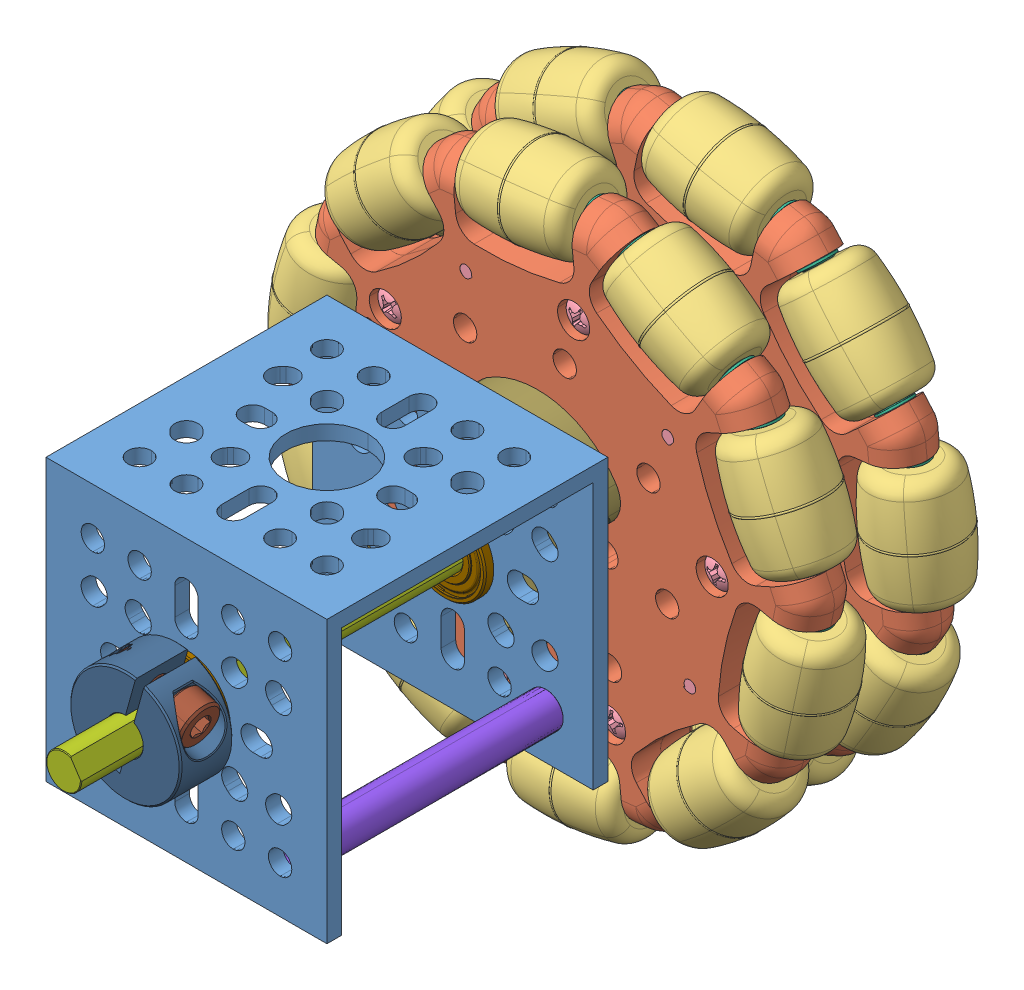
SolidWorks assembly directionOmni, configuration Défaut. Lengths in mm.
Overall size (122.26 122.26 115.2).
108 component instances, 14 part files, 27 mates.
Components (placement in the parent):
- 1120-0001-0048 u1-1: 1120-0001-0048 u1 [Défaut] at (-19.9494 20.1498 48) x (0 0 1) z (0 1 0) size (48 48 48)
- 3604-0014-0096 assembly-1: 3604-0014-0096 assembly [Défaut] at (47.7344 -1.1434 -33.9164) x (0.978755 -0.205033 0) z (-0.205033 -0.978755 0) size (103.42 20.4 102.56)
  - 3604-0014-0096 assembly.STEP-1: 3604-0014-0096 assembly.STEP [Défaut] at origin size (103.42 20.4 102.56)
    - 3604-0014-0096 wheel half.STEP-1: 3604-0014-0096 wheel half.STEP [Défaut] at (-42.7133 16.9164 9.1591) size (92.38 5.01 87.87)
    - 595671 omni wheel roller.STEP-1: 595671 omni wheel roller.STEP [Défaut] at (-66.8586 21.9164 42.3923) x (0.345492 -0.809017 -0.475528) z (-0.809017 0 -0.587785) size (14.61 14.61 19.05)
    - 364 omni wheel screw_99461A110.STEP-1: 364 omni wheel screw_99461A110.STEP [Défaut] at (-66.9838 22.9164 26.7926) x (-0.972951 0 0.231012) z (0 -1 0) size (5.22 5.22 9.61)
    - 3604-0014-0096 shaft.STEP-1: 3604-0014-0096 shaft.STEP [Défaut] at (-77.1615 21.9164 34.9068) x (0.587659 0.020713 -0.808843) z (0.012175 -0.999785 -0.016757) size (3.17 25.47 3.17)
    - 595671 omni wheel bushing.STEP-1: 595671 omni wheel bushing.STEP [Défaut] at (-66.8586 21.9164 42.3923) x (-0.041473 -0.997508 0.057082) z (-0.809017 0 -0.587785) size (5.61 5.61 20.15)
    - 364 omni wheel screw_99461A110.STEP-2: 364 omni wheel screw_99461A110.STEP [Défaut] at (-66.9838 22.9164 -8.4745) x (-0.520363 0 -0.853945) z (0 -1 0) size (5.22 5.22 9.61)
    - 364 omni wheel screw_99461A110.STEP-3: 364 omni wheel screw_99461A110.STEP [Défaut] at (-33.4428 22.9164 -19.3726) x (0.651349 0 -0.758779) z (0 -1 0) size (5.22 5.22 9.61)
    - 364 omni wheel screw_99461A110.STEP-4: 364 omni wheel screw_99461A110.STEP [Défaut] at (-12.7133 22.9164 9.1591) x (0.922919 0 0.384994) z (0 -1 0) size (5.22 5.22 9.61)
    - 364 omni wheel screw_99461A110.STEP-5: 364 omni wheel screw_99461A110.STEP [Défaut] at (-33.4428 22.9164 37.6908) x (-0.080953 0 0.996718) z (0 -1 0) size (5.22 5.22 9.61)
    - 3604-0014-0096 shaft.STEP-2: 3604-0014-0096 shaft.STEP [Défaut] at (-85.7166 21.9164 9.7413) x (0.950852 0.020713 -0.308951) z (0.019699 -0.999785 -0.006401) size (3.17 25.47 3.17)
    - 3604-0014-0096 shaft.STEP-3: 3604-0014-0096 shaft.STEP [Défaut] at (-77.846 21.9164 -15.6466) x (0.950852 0.020713 0.308951) z (0.019699 -0.999785 0.006401) size (3.17 25.47 3.17)
    - 3604-0014-0096 shaft.STEP-4: 3604-0014-0096 shaft.STEP [Défaut] at (-56.5558 21.9164 -31.5596) x (0.587659 0.020713 0.808843) z (0.012175 -0.999785 0.016757) size (3.17 25.47 3.17)
    - 3604-0014-0096 shaft.STEP-5: 3604-0014-0096 shaft.STEP [Défaut] at (-29.9783 21.9164 -31.9195) x (0 0.020713 0.999785) z (0 -0.999785 0.020713) size (3.17 25.47 3.17)
    - 3604-0014-0096 shaft.STEP-6: 3604-0014-0096 shaft.STEP [Défaut] at (-8.2651 21.9164 -16.5887) x (-0.587659 0.020713 0.808843) z (-0.012175 -0.999785 0.016757) size (3.17 25.47 3.17)
    - 3604-0014-0096 shaft.STEP-7: 3604-0014-0096 shaft.STEP [Défaut] at (0.29 21.9164 8.5768) x (-0.950852 0.020713 0.308951) z (-0.019699 -0.999785 0.006401) size (3.17 25.47 3.17)
    - 3604-0014-0096 shaft.STEP-8: 3604-0014-0096 shaft.STEP [Défaut] at (-7.5806 21.9164 33.9647) x (-0.950852 0.020713 -0.308951) z (-0.019699 -0.999785 -0.006401) size (3.17 25.47 3.17)
    - 3604-0014-0096 shaft.STEP-9: 3604-0014-0096 shaft.STEP [Défaut] at (-28.8708 21.9164 49.8777) x (-0.587659 0.020713 -0.808843) z (-0.012175 -0.999785 -0.016757) size (3.17 25.47 3.17)
    - 3604-0014-0096 shaft.STEP-10: 3604-0014-0096 shaft.STEP [Défaut] at (-55.4483 21.9164 50.2376) x (0 0.020713 -0.999785) z (0 -0.999785 -0.020713) size (3.17 25.47 3.17)
    - 595671 omni wheel bushing.STEP-2: 595671 omni wheel bushing.STEP [Défaut] at (-81.7813 21.9164 21.853) x (-0.067104 -0.997508 0.021803) z (-0.309017 0 -0.951057) size (5.61 5.61 20.15)
    - 595671 omni wheel bushing.STEP-3: 595671 omni wheel bushing.STEP [Défaut] at (-81.7813 21.9164 -3.5349) x (-0.067104 -0.997508 -0.021803) z (0.309017 0 -0.951057) size (5.61 5.61 20.15)
    - 595671 omni wheel bushing.STEP-4: 595671 omni wheel bushing.STEP [Défaut] at (-66.8586 21.9164 -24.0742) x (-0.041473 -0.997508 -0.057082) z (0.809017 0 -0.587785) size (5.61 5.61 20.15)
    - 595671 omni wheel bushing.STEP-5: 595671 omni wheel bushing.STEP [Défaut] at (-42.7133 21.9164 -31.9195) x (0 -0.997508 -0.070558) z (1 0 0) size (5.61 5.61 20.15)
    - 595671 omni wheel bushing.STEP-6: 595671 omni wheel bushing.STEP [Défaut] at (-18.5679 21.9164 -24.0742) x (0.041473 -0.997508 -0.057082) z (0.809017 0 0.587785) size (5.61 5.61 20.15)
    - 595671 omni wheel bushing.STEP-7: 595671 omni wheel bushing.STEP [Défaut] at (-3.6453 21.9164 -3.5349) x (0.067104 -0.997508 -0.021803) z (0.309017 0 0.951057) size (5.61 5.61 20.15)
    - 595671 omni wheel bushing.STEP-8: 595671 omni wheel bushing.STEP [Défaut] at (-3.6453 21.9164 21.853) x (0.067104 -0.997508 0.021803) z (-0.309017 0 0.951057) size (5.61 5.61 20.15)
    - 595671 omni wheel bushing.STEP-9: 595671 omni wheel bushing.STEP [Défaut] at (-18.5679 21.9164 42.3923) x (0.041473 -0.997508 0.057082) z (-0.809017 0 0.587785) size (5.61 5.61 20.15)
    - 595671 omni wheel bushing.STEP-10: 595671 omni wheel bushing.STEP [Défaut] at (-42.7133 21.9164 50.2376) x (0 -0.997508 0.070558) z (-1 0 0) size (5.61 5.61 20.15)
    - 595671 omni wheel roller.STEP-2: 595671 omni wheel roller.STEP [Défaut] at (-81.7813 21.9164 21.853) x (0.559017 -0.809017 -0.181636) z (-0.309017 0 -0.951057) size (14.61 14.61 19.05)
    - 595671 omni wheel roller.STEP-3: 595671 omni wheel roller.STEP [Défaut] at (-81.7813 21.9164 -3.5349) x (0.559017 -0.809017 0.181636) z (0.309017 0 -0.951057) size (14.61 14.61 19.05)
    - 595671 omni wheel roller.STEP-4: 595671 omni wheel roller.STEP [Défaut] at (-66.8586 21.9164 -24.0742) x (0.345492 -0.809017 0.475528) z (0.809017 0 -0.587785) size (14.61 14.61 19.05)
    - 595671 omni wheel roller.STEP-5: 595671 omni wheel roller.STEP [Défaut] at (-42.7133 21.9164 -31.9195) x (0 -0.809017 0.587785) z (1 0 0) size (14.61 14.61 19.05)
    - 595671 omni wheel roller.STEP-6: 595671 omni wheel roller.STEP [Défaut] at (-18.5679 21.9164 -24.0742) x (-0.345492 -0.809017 0.475528) z (0.809017 0 0.587785) size (14.61 14.61 19.05)
    - 595671 omni wheel roller.STEP-7: 595671 omni wheel roller.STEP [Défaut] at (-3.6453 21.9164 -3.5349) x (-0.559017 -0.809017 0.181636) z (0.309017 0 0.951057) size (14.61 14.61 19.05)
    - 595671 omni wheel roller.STEP-8: 595671 omni wheel roller.STEP [Défaut] at (-3.6453 21.9164 21.853) x (-0.559017 -0.809017 -0.181636) z (-0.309017 0 0.951057) size (14.61 14.61 19.05)
    - 595671 omni wheel roller.STEP-9: 595671 omni wheel roller.STEP [Défaut] at (-18.5679 21.9164 42.3923) x (-0.345492 -0.809017 -0.475528) z (-0.809017 0 0.587785) size (14.61 14.61 19.05)
    - 595671 omni wheel roller.STEP-10: 595671 omni wheel roller.STEP [Défaut] at (-42.7133 21.9164 50.2376) x (0 -0.809017 -0.587785) z (-1 0 0) size (14.61 14.61 19.05)
    - 3604-0014-0096 wheel half.STEP-2: 3604-0014-0096 wheel half.STEP [Défaut] at (-42.7133 26.9164 9.1591) x (-1 0 0) z (0 0 1) size (92.38 5.01 87.87)
    - 364 omni wheel screw_99461A110.STEP-6: 364 omni wheel screw_99461A110.STEP [Défaut] at (-51.9838 20.9164 37.6908) x (-0.514694 0 0.857374) z (0 1 0) size (5.22 5.22 9.61)
    - 364 omni wheel screw_99461A110.STEP-7: 364 omni wheel screw_99461A110.STEP [Défaut] at (-18.4428 20.9164 26.7926) x (0.656361 0 0.754447) z (0 1 0) size (5.22 5.22 9.61)
    - 364 omni wheel screw_99461A110.STEP-8: 364 omni wheel screw_99461A110.STEP [Défaut] at (-18.4428 20.9164 -8.4745) x (0.920348 0 -0.3911) z (0 1 0) size (5.22 5.22 9.61)
    - 364 omni wheel screw_99461A110.STEP-9: 364 omni wheel screw_99461A110.STEP [Défaut] at (-51.9838 20.9164 -19.3726) x (-0.087555 0 -0.99616) z (0 1 0) size (5.22 5.22 9.61)
    - 364 omni wheel screw_99461A110.STEP-10: 364 omni wheel screw_99461A110.STEP [Défaut] at (-72.7133 20.9164 9.1591) x (-0.97446 0 -0.22456) z (0 1 0) size (5.22 5.22 9.61)
- 3604-0014-0096 assembly-2: 3604-0014-0096 assembly [Défaut] at (4.2575 -45.034 -14.9164) x (-0.205033 -0.978755 0) z (-0.978755 0.205033 0) size (103.42 20.4 102.56)
  - 3604-0014-0096 assembly.STEP-1: 3604-0014-0096 assembly.STEP [Défaut] at origin size (103.42 20.4 102.56)
    - 3604-0014-0096 wheel half.STEP-1: 3604-0014-0096 wheel half.STEP [Défaut] at (-42.7133 16.9164 9.1591) size (92.38 5.01 87.87)
    - 595671 omni wheel roller.STEP-1: 595671 omni wheel roller.STEP [Défaut] at (-66.8586 21.9164 42.3923) x (0.345492 -0.809017 -0.475528) z (-0.809017 0 -0.587785) size (14.61 14.61 19.05)
    - 364 omni wheel screw_99461A110.STEP-1: 364 omni wheel screw_99461A110.STEP [Défaut] at (-66.9838 22.9164 26.7926) x (-0.972951 0 0.231012) z (0 -1 0) size (5.22 5.22 9.61)
    - 3604-0014-0096 shaft.STEP-1: 3604-0014-0096 shaft.STEP [Défaut] at (-77.1615 21.9164 34.9068) x (0.587659 0.020713 -0.808843) z (0.012175 -0.999785 -0.016757) size (3.17 25.47 3.17)
    - 595671 omni wheel bushing.STEP-1: 595671 omni wheel bushing.STEP [Défaut] at (-66.8586 21.9164 42.3923) x (-0.041473 -0.997508 0.057082) z (-0.809017 0 -0.587785) size (5.61 5.61 20.15)
    - 364 omni wheel screw_99461A110.STEP-2: 364 omni wheel screw_99461A110.STEP [Défaut] at (-66.9838 22.9164 -8.4745) x (-0.520363 0 -0.853945) z (0 -1 0) size (5.22 5.22 9.61)
    - 364 omni wheel screw_99461A110.STEP-3: 364 omni wheel screw_99461A110.STEP [Défaut] at (-33.4428 22.9164 -19.3726) x (0.651349 0 -0.758779) z (0 -1 0) size (5.22 5.22 9.61)
    - 364 omni wheel screw_99461A110.STEP-4: 364 omni wheel screw_99461A110.STEP [Défaut] at (-12.7133 22.9164 9.1591) x (0.922919 0 0.384994) z (0 -1 0) size (5.22 5.22 9.61)
    - 364 omni wheel screw_99461A110.STEP-5: 364 omni wheel screw_99461A110.STEP [Défaut] at (-33.4428 22.9164 37.6908) x (-0.080953 0 0.996718) z (0 -1 0) size (5.22 5.22 9.61)
    - 3604-0014-0096 shaft.STEP-2: 3604-0014-0096 shaft.STEP [Défaut] at (-85.7166 21.9164 9.7413) x (0.950852 0.020713 -0.308951) z (0.019699 -0.999785 -0.006401) size (3.17 25.47 3.17)
    - 3604-0014-0096 shaft.STEP-3: 3604-0014-0096 shaft.STEP [Défaut] at (-77.846 21.9164 -15.6466) x (0.950852 0.020713 0.308951) z (0.019699 -0.999785 0.006401) size (3.17 25.47 3.17)
    - 3604-0014-0096 shaft.STEP-4: 3604-0014-0096 shaft.STEP [Défaut] at (-56.5558 21.9164 -31.5596) x (0.587659 0.020713 0.808843) z (0.012175 -0.999785 0.016757) size (3.17 25.47 3.17)
    - 3604-0014-0096 shaft.STEP-5: 3604-0014-0096 shaft.STEP [Défaut] at (-29.9783 21.9164 -31.9195) x (0 0.020713 0.999785) z (0 -0.999785 0.020713) size (3.17 25.47 3.17)
    - 3604-0014-0096 shaft.STEP-6: 3604-0014-0096 shaft.STEP [Défaut] at (-8.2651 21.9164 -16.5887) x (-0.587659 0.020713 0.808843) z (-0.012175 -0.999785 0.016757) size (3.17 25.47 3.17)
    - 3604-0014-0096 shaft.STEP-7: 3604-0014-0096 shaft.STEP [Défaut] at (0.29 21.9164 8.5768) x (-0.950852 0.020713 0.308951) z (-0.019699 -0.999785 0.006401) size (3.17 25.47 3.17)
    - 3604-0014-0096 shaft.STEP-8: 3604-0014-0096 shaft.STEP [Défaut] at (-7.5806 21.9164 33.9647) x (-0.950852 0.020713 -0.308951) z (-0.019699 -0.999785 -0.006401) size (3.17 25.47 3.17)
    - 3604-0014-0096 shaft.STEP-9: 3604-0014-0096 shaft.STEP [Défaut] at (-28.8708 21.9164 49.8777) x (-0.587659 0.020713 -0.808843) z (-0.012175 -0.999785 -0.016757) size (3.17 25.47 3.17)
    - 3604-0014-0096 shaft.STEP-10: 3604-0014-0096 shaft.STEP [Défaut] at (-55.4483 21.9164 50.2376) x (0 0.020713 -0.999785) z (0 -0.999785 -0.020713) size (3.17 25.47 3.17)
    - 595671 omni wheel bushing.STEP-2: 595671 omni wheel bushing.STEP [Défaut] at (-81.7813 21.9164 21.853) x (-0.067104 -0.997508 0.021803) z (-0.309017 0 -0.951057) size (5.61 5.61 20.15)
    - 595671 omni wheel bushing.STEP-3: 595671 omni wheel bushing.STEP [Défaut] at (-81.7813 21.9164 -3.5349) x (-0.067104 -0.997508 -0.021803) z (0.309017 0 -0.951057) size (5.61 5.61 20.15)
    - 595671 omni wheel bushing.STEP-4: 595671 omni wheel bushing.STEP [Défaut] at (-66.8586 21.9164 -24.0742) x (-0.041473 -0.997508 -0.057082) z (0.809017 0 -0.587785) size (5.61 5.61 20.15)
    - 595671 omni wheel bushing.STEP-5: 595671 omni wheel bushing.STEP [Défaut] at (-42.7133 21.9164 -31.9195) x (0 -0.997508 -0.070558) z (1 0 0) size (5.61 5.61 20.15)
    - 595671 omni wheel bushing.STEP-6: 595671 omni wheel bushing.STEP [Défaut] at (-18.5679 21.9164 -24.0742) x (0.041473 -0.997508 -0.057082) z (0.809017 0 0.587785) size (5.61 5.61 20.15)
    - 595671 omni wheel bushing.STEP-7: 595671 omni wheel bushing.STEP [Défaut] at (-3.6453 21.9164 -3.5349) x (0.067104 -0.997508 -0.021803) z (0.309017 0 0.951057) size (5.61 5.61 20.15)
    - 595671 omni wheel bushing.STEP-8: 595671 omni wheel bushing.STEP [Défaut] at (-3.6453 21.9164 21.853) x (0.067104 -0.997508 0.021803) z (-0.309017 0 0.951057) size (5.61 5.61 20.15)
    - 595671 omni wheel bushing.STEP-9: 595671 omni wheel bushing.STEP [Défaut] at (-18.5679 21.9164 42.3923) x (0.041473 -0.997508 0.057082) z (-0.809017 0 0.587785) size (5.61 5.61 20.15)
    - 595671 omni wheel bushing.STEP-10: 595671 omni wheel bushing.STEP [Défaut] at (-42.7133 21.9164 50.2376) x (0 -0.997508 0.070558) z (-1 0 0) size (5.61 5.61 20.15)
    - 595671 omni wheel roller.STEP-2: 595671 omni wheel roller.STEP [Défaut] at (-81.7813 21.9164 21.853) x (0.559017 -0.809017 -0.181636) z (-0.309017 0 -0.951057) size (14.61 14.61 19.05)
    - 595671 omni wheel roller.STEP-3: 595671 omni wheel roller.STEP [Défaut] at (-81.7813 21.9164 -3.5349) x (0.559017 -0.809017 0.181636) z (0.309017 0 -0.951057) size (14.61 14.61 19.05)
    - 595671 omni wheel roller.STEP-4: 595671 omni wheel roller.STEP [Défaut] at (-66.8586 21.9164 -24.0742) x (0.345492 -0.809017 0.475528) z (0.809017 0 -0.587785) size (14.61 14.61 19.05)
    - 595671 omni wheel roller.STEP-5: 595671 omni wheel roller.STEP [Défaut] at (-42.7133 21.9164 -31.9195) x (0 -0.809017 0.587785) z (1 0 0) size (14.61 14.61 19.05)
    - 595671 omni wheel roller.STEP-6: 595671 omni wheel roller.STEP [Défaut] at (-18.5679 21.9164 -24.0742) x (-0.345492 -0.809017 0.475528) z (0.809017 0 0.587785) size (14.61 14.61 19.05)
    - 595671 omni wheel roller.STEP-7: 595671 omni wheel roller.STEP [Défaut] at (-3.6453 21.9164 -3.5349) x (-0.559017 -0.809017 0.181636) z (0.309017 0 0.951057) size (14.61 14.61 19.05)
    - 595671 omni wheel roller.STEP-8: 595671 omni wheel roller.STEP [Défaut] at (-3.6453 21.9164 21.853) x (-0.559017 -0.809017 -0.181636) z (-0.309017 0 0.951057) size (14.61 14.61 19.05)
    - 595671 omni wheel roller.STEP-9: 595671 omni wheel roller.STEP [Défaut] at (-18.5679 21.9164 42.3923) x (-0.345492 -0.809017 -0.475528) z (-0.809017 0 0.587785) size (14.61 14.61 19.05)
    - 595671 omni wheel roller.STEP-10: 595671 omni wheel roller.STEP [Défaut] at (-42.7133 21.9164 50.2376) x (0 -0.809017 -0.587785) z (-1 0 0) size (14.61 14.61 19.05)
    - 3604-0014-0096 wheel half.STEP-2: 3604-0014-0096 wheel half.STEP [Défaut] at (-42.7133 26.9164 9.1591) x (-1 0 0) z (0 0 1) size (92.38 5.01 87.87)
    - 364 omni wheel screw_99461A110.STEP-6: 364 omni wheel screw_99461A110.STEP [Défaut] at (-51.9838 20.9164 37.6908) x (-0.514694 0 0.857374) z (0 1 0) size (5.22 5.22 9.61)
    - 364 omni wheel screw_99461A110.STEP-7: 364 omni wheel screw_99461A110.STEP [Défaut] at (-18.4428 20.9164 26.7926) x (0.656361 0 0.754447) z (0 1 0) size (5.22 5.22 9.61)
    - 364 omni wheel screw_99461A110.STEP-8: 364 omni wheel screw_99461A110.STEP [Défaut] at (-18.4428 20.9164 -8.4745) x (0.920348 0 -0.3911) z (0 1 0) size (5.22 5.22 9.61)
    - 364 omni wheel screw_99461A110.STEP-9: 364 omni wheel screw_99461A110.STEP [Défaut] at (-51.9838 20.9164 -19.3726) x (-0.087555 0 -0.99616) z (0 1 0) size (5.22 5.22 9.61)
    - 364 omni wheel screw_99461A110.STEP-10: 364 omni wheel screw_99461A110.STEP [Défaut] at (-72.7133 20.9164 9.1591) x (-0.97446 0 -0.22456) z (0 1 0) size (5.22 5.22 9.61)
- 2101-0006-0100 essieuCourt-1: 2101-0006-0100 essieuCourt [Défaut] at (4.0506 -1.3502 -7) x (0.547104 -0.837065 0) z (-0.837065 -0.547104 0) size (6 100 5.5)
- 1501-0006-0430 renfort-1: 1501-0006-0430 renfort [Défaut] at (-11.9494 -17.3502 48) x (0 1 0) z (1 0 0) size (5.95 43.01 5.95)
- 1501-0006-0430 renfort-2: 1501-0006-0430 renfort [Défaut] at (20.0506 -17.3502 48) x (1 0 0) z (0 -1 0) size (5.95 43.01 5.95)
- 1611-0514-0006-1: 1611-0514-0006 [Défaut] at (4.0506 -1.3502 28) x (-0.582956 0.812503 0) z (-0.812503 -0.582956 0) size (15 5 15)
- 1611-0514-0006-2: 1611-0514-0006 [Défaut] at (4.0506 -1.3502 68) x (0.993873 0.110524 0) z (0.110524 -0.993873 0) size (15 5 15)
- 2910-0919-0006 assembly collet-1: 2910-0919-0006 assembly collet [Défaut] at (-4.3426 32.9112 -1.9796) x (0.251082 0.967966 0) z (0.967966 -0.251082 0) size (19 9.89 19.83)
  - 2910-0919-0006 assembly.STEP-1: 2910-0919-0006 assembly.STEP [Défaut] at origin size (19 9.89 19.83)
    - 2910-0919-0006.STEP-1: 2910-0919-0006.STEP [Défaut] at (-31.0565 -0.5204 16.7268) size (19 9.5 18.97)
    - 2800-0004-0010_90128A207.STEP-1: 2800-0004-0010_90128A207.STEP [Défaut] at (-24.2865 -0.5204 11.2868) x (0 -0.807243 -0.59022) z (1 0 0) size (7 7 14.01)
- 1309-0016-1006 assembly-1: 1309-0016-1006 assembly [Défaut] at (21.7473 -5.6475 7.2264) x (0.978755 -0.205033 0) z (0 0 1) size (28.36 32 10.95)
  - 1309-0016-1006 assembly.STEP-1: 1309-0016-1006 assembly.STEP [Défaut] at origin size (28.36 32 10.95)
    - 1309-0016-1006.STEP-1: 1309-0016-1006.STEP [Défaut] at (-18.2019 0.5776 8.7736) size (25.38 32 10)
    - 2800-0004-0014_90128A207.STEP-1: 2800-0004-0014_90128A207.STEP [Défaut] at (-16.149 11.6963 8.7736) x (0.5 -0.5 -0.707107) z (0.707107 0.707107 0) size (7 7 18.01)
    - 2800-0004-0014_90128A207.STEP-2: 2800-0004-0014_90128A207.STEP [Défaut] at (-20.2547 -10.5411 8.7736) x (-0.5 0.5 -0.707107) z (-0.707107 -0.707107 0) size (7 7 18.01)
- 2910-0919-0006 assembly collet-2: 2910-0919-0006 assembly collet [Défaut] at (-21.4149 23.0588 77.4796) x (-0.963724 0.266899 0) z (-0.266899 -0.963724 0) size (19 9.89 19.83)
  - 2910-0919-0006 assembly.STEP-1: 2910-0919-0006 assembly.STEP [Défaut] at origin size (19 9.89 19.83)
    - 2910-0919-0006.STEP-1: 2910-0919-0006.STEP [Défaut] at (-31.0565 -0.5204 16.7268) size (19 9.5 18.97)
    - 2800-0004-0010_90128A207.STEP-1: 2800-0004-0010_90128A207.STEP [Défaut] at (-24.2865 -0.5204 11.2868) x (0 -0.807243 -0.59022) z (1 0 0) size (7 7 14.01)
- 2807-0609-1000-1: 2807-0609-1000 [Défaut] at (4.0506 -1.3502 22) x (1 0 0) z (0 -1 0) size (9 1 9)
Mates (geometry in assembly coordinates):
- Coaxiale2: concentric: cylinder of 3604-0014-0096 assembly-1/3604-0014-0096 assembly.STEP-1/3604-0014-0096 wheel half.STEP-1 through (4.0506 -1.3502 -12) axis (0 0 -1) radius 7; cylinder of 2101-0006-0100 essieuCourt-1 through (4.0506 -1.3502 93) axis (0 0 -1) radius 3
- Coaxiale3: concentric: cylinder of 1120-0001-0048 u1-1 through (4.0506 -1.3502 34) axis (0 0 -1) radius 7; cylinder of 2101-0006-0100 essieuCourt-1 through (4.0506 -1.3502 93) axis (0 0 -1) radius 3
- Coaxiale4: concentric: cylinder of 3604-0014-0096 assembly-2/3604-0014-0096 assembly.STEP-1/3604-0014-0096 wheel half.STEP-1 through (4.0506 -1.3502 7) axis (0 0 -1) radius 7; cylinder of 2101-0006-0100 essieuCourt-1 through (4.0506 -1.3502 93) axis (0 0 -1) radius 3
- Coaxiale5: concentric: cylinder of 3604-0014-0096 assembly-1/3604-0014-0096 assembly.STEP-1/3604-0014-0096 wheel half.STEP-1 through (-5.9942 -7.9155 -12) axis (0 0 -1) radius 2; cylinder of 3604-0014-0096 assembly-2/3604-0014-0096 assembly.STEP-1/3604-0014-0096 wheel half.STEP-1 through (-5.9942 -7.9155 7) axis (0 0 -1) radius 2
- Coaxiale7: concentric: cylinder of 2101-0006-0100 essieuCourt-1 through (4.0506 -1.3502 93) axis (0 0 -1) radius 3; cylinder of 2910-0919-0006 assembly collet-1/2910-0919-0006 assembly.STEP-1/2910-0919-0006.STEP-1 through (4.0506 -1.3502 2) axis (0 0 -1) radius 3
- Coïncidente1: coincident: plane of 3604-0014-0096 assembly-1/3604-0014-0096 assembly.STEP-1/3604-0014-0096 wheel half.STEP-2 through (4.0506 -1.3502 -7) normal (0 0 1); plane of 2910-0919-0006 assembly collet-1/2910-0919-0006 assembly.STEP-1/2910-0919-0006.STEP-1 through (4.0506 -1.3502 -7) normal (0 0 -1)
- Coïncidente2: coincident: plane of 3604-0014-0096 assembly-2/3604-0014-0096 assembly.STEP-1/3604-0014-0096 wheel half.STEP-1 through (4.0506 -1.3502 2) normal (0 0 -1); plane of 2910-0919-0006 assembly collet-1/2910-0919-0006 assembly.STEP-1/2910-0919-0006.STEP-1 through (4.0506 -1.3502 2) normal (0 0 1)
- Coaxiale8: concentric: cylinder of 2101-0006-0100 essieuCourt-1 through (4.0506 -1.3502 93) axis (0 0 -1) radius 3; cylinder of 1611-0514-0006-1 through (4.0506 -1.3502 28) axis (0 0 -1) radius 3
- Coïncidente6: coincident: plane of 1120-0001-0048 u1-1 through (28.0506 -25.3502 24) normal (0 0 -1); plane of 1611-0514-0006-1 through (4.0506 -1.3502 24) normal (0 0 1)
- Coaxiale10: concentric: cylinder of 2101-0006-0100 essieuCourt-1 through (4.0506 -1.3502 93) axis (0 0 -1) radius 3; cylinder of 2807-0609-1000-1 through (4.0506 -1.3502 23) axis (0 0 -1) radius 3
- Coïncidente7: coincident: plane of 1611-0514-0006-1 through (4.0506 -1.3502 23) normal (0 0 -1); plane of 2807-0609-1000-1 through (4.0506 -1.3502 23) normal (0 0 1)
- Coaxiale11: concentric: cylinder of 2101-0006-0100 essieuCourt-1 through (4.0506 -1.3502 93) axis (0 0 -1) radius 3; cylinder of 1611-0514-0006-2 through (4.0506 -1.3502 68) axis (0 0 1) radius 3
- Coïncidente9: coincident: plane of 1120-0001-0048 u1-1 through (28.0506 -25.3502 72) normal (0 0 1); plane of 1611-0514-0006-2 through (4.0506 -1.3502 72) normal (0 0 -1)
- Coaxiale17: concentric: cylinder of 2101-0006-0100 essieuCourt-1 through (4.0506 -1.3502 93) axis (0 0 -1) radius 3; cylinder of 2910-0919-0006 assembly collet-2/2910-0919-0006 assembly.STEP-1/2910-0919-0006.STEP-1 through (4.0506 -1.3502 73.5) axis (0 0 1) radius 3
- Coïncidente12: coincident: plane of 1611-0514-0006-2 through (4.0506 -1.3502 73) normal (0 0 1); plane of 2910-0919-0006 assembly collet-2/2910-0919-0006 assembly.STEP-1/2910-0919-0006.STEP-1 through (4.0506 -1.3502 73) normal (0 0 -1)
- Coïncidente13: coincident: plane of 1120-0001-0048 u1-1 through (28.0506 20.1498 69.5) normal (0 0 -1); plane of 1501-0006-0430 renfort-2 through (20.0506 -17.3502 69.5) normal (0 0 1)
- Coaxiale18: concentric: cylinder of 1120-0001-0048 u1-1 through (20.0506 -17.3502 62) axis (0 0 1) radius 2; cylinder of 1501-0006-0430 renfort-2 through (20.0506 -17.3502 69.5) axis (0 0 -1) radius 2.975
- Coïncidente14: coincident: plane of 1120-0001-0048 u1-1 through (28.0506 20.1498 69.5) normal (0 0 -1); plane of 1501-0006-0430 renfort-1 through (-11.9494 -17.3502 69.5) normal (0 0 1)
- Coaxiale19: concentric: cylinder of 1120-0001-0048 u1-1 through (-11.9494 -17.3502 62) axis (0 0 1) radius 2; cylinder of 1501-0006-0430 renfort-1 through (-11.9494 -17.3502 69.5) axis (0 0 -1) radius 2.975
- Coaxiale20: concentric: cylinder of 2101-0006-0100 essieuCourt-1 through (4.0506 -1.3502 93) axis (0 0 -1) radius 3; cylinder of 1309-0016-1006 assembly-1/1309-0016-1006 assembly.STEP-1/1309-0016-1006.STEP-1 through (4.0506 -1.3502 11.7495) axis (0 0 1) radius 3
- Parallèle2: parallel: plane of 2101-0006-0100 essieuCourt-1 through (6.1433 0.0176 93) normal (0.837065 0.547104 0); plane of 1309-0016-1006 assembly-1/1309-0016-1006 assembly.STEP-1/1309-0016-1006.STEP-1 through (6.1265 0.0066 11.7495) normal (-0.837065 -0.547104 0)
- Coïncidente16: coincident: plane of 1309-0016-1006 assembly-1/1309-0016-1006 assembly.STEP-1/1309-0016-1006.STEP-1 through (4.0506 -1.3502 22) normal (0 0 1); plane of 2807-0609-1000-1 through (4.0506 -1.3502 22) normal (0 0 -1)
- Coaxiale21: concentric: cylinder of 3604-0014-0096 assembly-2/3604-0014-0096 assembly.STEP-1/3604-0014-0096 wheel half.STEP-2 through (4.0506 -1.3502 7) axis (0 0 1) radius 7; cylinder of 2101-0006-0100 essieuCourt-1 through (4.0506 -1.3502 93) axis (0 0 -1) radius 3
- Coaxiale22: concentric: cylinder of 3604-0014-0096 assembly-2/3604-0014-0096 assembly.STEP-1/3604-0014-0096 wheel half.STEP-2 through (4.0506 -1.3502 7) axis (0 0 1) radius 7; cylinder of 2101-0006-0100 essieuCourt-1 through (4.0506 -1.3502 93) axis (0 0 -1) radius 3
- Coaxiale23: concentric: circle of 3604-0014-0096 assembly-2/3604-0014-0096 assembly.STEP-1/3604-0014-0096 wheel half.STEP-2; circle of 1309-0016-1006 assembly-1/1309-0016-1006 assembly.STEP-1/1309-0016-1006.STEP-1
- Coïncidente18: coincident: plane of 3604-0014-0096 assembly-2/3604-0014-0096 assembly.STEP-1/3604-0014-0096 wheel half.STEP-2 through (4.0506 -1.3502 12) normal (0 0 1); plane of 1309-0016-1006 assembly-1/1309-0016-1006 assembly.STEP-1/1309-0016-1006.STEP-1 through (4.0506 -1.3502 12) normal (0 0 -1)
- Coïncidente19: coincident: plane of 2101-0006-0100 essieuCourt-1 through (4.0506 -1.3502 -7) normal (0 0 -1); plane of 2910-0919-0006 assembly collet-1/2910-0919-0006 assembly.STEP-1/2910-0919-0006.STEP-1 through (4.0506 -1.3502 -7) normal (0 0 -1)
